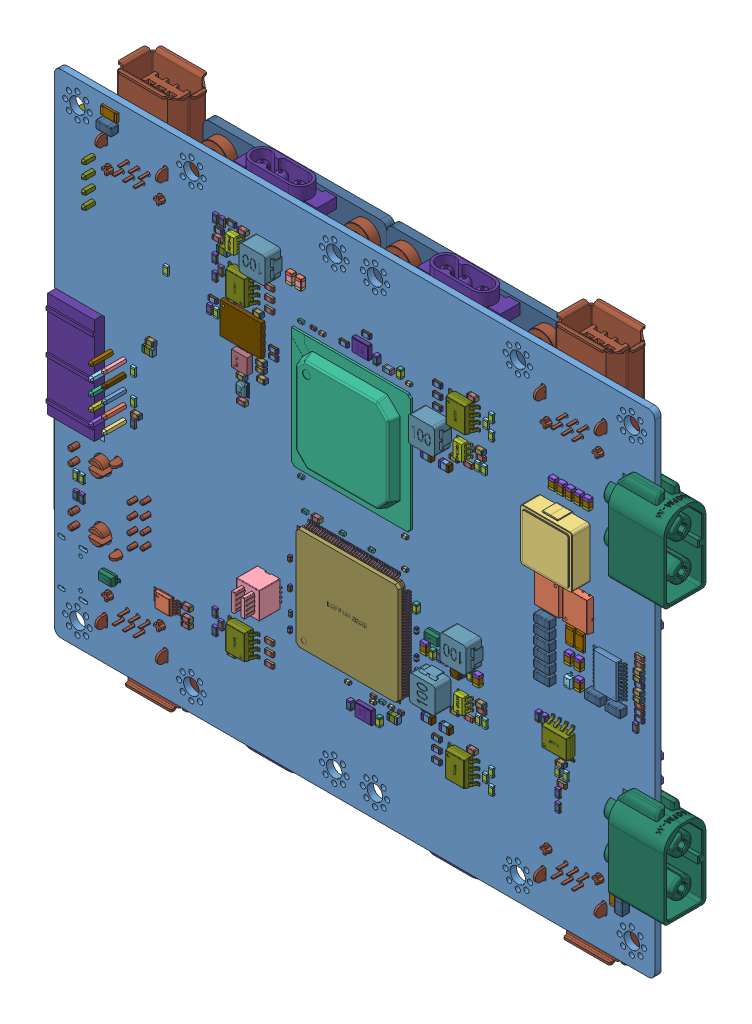
SolidWorks assembly Mother  Board, configuration 默认. Lengths in mm. (continued)
Components (placement in the parent): (continued)
- Mother  Board.step-1: Mother  Board.step [默认] at origin size (122.6 102.08 21) (continued)
  - R56.step-1: R56.step [默认] at origin size (0.5 1 0.35)
    - 5993847584.step-1: 5993847584.step [默认] at (46.4669 57.4279 -1.2164) x (0 -1 0) z (0 0 -1) size (1 0.5 0.35)
      - Terminal-11.step-1: Terminal-11.step [默认] at (-0.5 -0.25 0) size (0.25 0.5 0.35)
        - Open_CASCADE_STEP_translator_6.8_20.2.1-25.step-1: Open_CASCADE_STEP_translator_6.8_20.2.1-25.step [默认] at origin size (0.25 0.5 0.35)
      - Terminal-11.step-2: Terminal-11.step [默认] at (0.5 0.25 0) x (-1 0 0) z (0 0 1) size (0.25 0.5 0.35)
        - Open_CASCADE_STEP_translator_6.8_20.2.1-25.step-1: Open_CASCADE_STEP_translator_6.8_20.2.1-25.step [默认] at origin size (0.25 0.5 0.35)
      - Mid_Body-26.step-1: Mid_Body-26.step [默认] at (-0.5 -0.25 0) size (0.93 0.5 0.28)
      - Mark-27.step-1: Mark-27.step [默认] at (-0.25 -0.25 0.315) size (0.5 0.5 0.03)
  - R55.step-1: R55.step [默认] at origin size (1 0.5 0.35)
    - 5993847504.step-1: 5993847504.step [默认] at (44.9669 62.9361 -1.2164) x (-1 0 0) z (0 0 -1) size (1 0.5 0.35)
      - Terminal-8.step-1: Terminal-8.step [默认] at (-0.5 -0.25 0) size (0.25 0.5 0.35)
        - Open_CASCADE_STEP_translator_6.8_20.2.1-16.step-1: Open_CASCADE_STEP_translator_6.8_20.2.1-16.step [默认] at origin size (0.25 0.5 0.35)
      - Terminal-8.step-2: Terminal-8.step [默认] at (0.5 0.25 0) x (-1 0 0) z (0 0 1) size (0.25 0.5 0.35)
        - Open_CASCADE_STEP_translator_6.8_20.2.1-16.step-1: Open_CASCADE_STEP_translator_6.8_20.2.1-16.step [默认] at origin size (0.25 0.5 0.35)
      - Mid_Body-17.step-1: Mid_Body-17.step [默认] at (-0.5 -0.25 0) size (0.93 0.5 0.28)
      - Mark-18.step-1: Mark-18.step [默认] at (-0.25 -0.25 0.315) size (0.5 0.5 0.03)
  - R54.step-1: R54.step [默认] at origin size (0.5 1 0.35)
    - 5993847584.step-1: 5993847584.step [默认] at (60.4669 57.4279 -1.2164) x (0 -1 0) z (0 0 -1) size (1 0.5 0.35)
      - Terminal-11.step-1: Terminal-11.step [默认] at (-0.5 -0.25 0) size (0.25 0.5 0.35)
        - Open_CASCADE_STEP_translator_6.8_20.2.1-25.step-1: Open_CASCADE_STEP_translator_6.8_20.2.1-25.step [默认] at origin size (0.25 0.5 0.35)
      - Terminal-11.step-2: Terminal-11.step [默认] at (0.5 0.25 0) x (-1 0 0) z (0 0 1) size (0.25 0.5 0.35)
        - Open_CASCADE_STEP_translator_6.8_20.2.1-25.step-1: Open_CASCADE_STEP_translator_6.8_20.2.1-25.step [默认] at origin size (0.25 0.5 0.35)
      - Mid_Body-26.step-1: Mid_Body-26.step [默认] at (-0.5 -0.25 0) size (0.93 0.5 0.28)
      - Mark-27.step-1: Mark-27.step [默认] at (-0.25 -0.25 0.315) size (0.5 0.5 0.03)
  - R53.step-1: R53.step [默认] at origin size (1.6 0.8 0.45)
    - 5993842144.step-1: 5993842144.step [默认] at (38.1001 64.5161 0) x (1 0 0) z (0 0 1) size (1.6 0.8 0.45)
      - Terminal-10.step-1: Terminal-10.step [默认] at (-0.8 -0.4 0) size (0.3 0.8 0.45)
        - Open_CASCADE_STEP_translator_6.8_21.2.1-22.step-1: Open_CASCADE_STEP_translator_6.8_21.2.1-22.step [默认] at origin size (0.3 0.8 0.45)
      - Terminal-10.step-2: Terminal-10.step [默认] at (0.8 0.4 0) x (-1 0 0) z (0 0 1) size (0.3 0.8 0.45)
        - Open_CASCADE_STEP_translator_6.8_21.2.1-22.step-1: Open_CASCADE_STEP_translator_6.8_21.2.1-22.step [默认] at origin size (0.3 0.8 0.45)
      - Mid_Body-23.step-1: Mid_Body-23.step [默认] at (-0.8 -0.4 0) size (1.51 0.8 0.36)
      - Mark-24.step-1: Mark-24.step [默认] at (-0.5 -0.4 0.405) size (1 0.8 0.05)
  - R52.step-1: R52.step [默认] at origin size (0.8 1.6 0.45)
    - 5993842864.step-1: 5993842864.step [默认] at (27.0509 65.1511 0) x (0 1 0) z (0 0 1) size (1.6 0.8 0.45)
      - Terminal-12.step-1: Terminal-12.step [默认] at (-0.8 -0.4 0) size (0.3 0.8 0.45)
        - Open_CASCADE_STEP_translator_6.8_21.2.1-28.step-1: Open_CASCADE_STEP_translator_6.8_21.2.1-28.step [默认] at origin size (0.3 0.8 0.45)
      - Terminal-12.step-2: Terminal-12.step [默认] at (0.8 0.4 0) x (-1 0 0) z (0 0 1) size (0.3 0.8 0.45)
        - Open_CASCADE_STEP_translator_6.8_21.2.1-28.step-1: Open_CASCADE_STEP_translator_6.8_21.2.1-28.step [默认] at origin size (0.3 0.8 0.45)
      - Mid_Body-29.step-1: Mid_Body-29.step [默认] at (-0.8 -0.4 0) size (1.51 0.8 0.36)
      - Mark-30.step-1: Mark-30.step [默认] at (-0.5 -0.4 0.405) size (1 0.8 0.05)
  - R51.step-1: R51.step [默认] at origin size (0.8 1.6 0.45)
    - 5993843024.step-1: 5993843024.step [默认] at (11.0491 38.7349 0) x (0 -1 0) z (0 0 1) size (1.6 0.8 0.45)
      - Terminal-13.step-1: Terminal-13.step [默认] at (-0.8 -0.4 0) size (0.3 0.8 0.45)
        - Open_CASCADE_STEP_translator_6.8_21.2.1-31.step-1: Open_CASCADE_STEP_translator_6.8_21.2.1-31.step [默认] at origin size (0.3 0.8 0.45)
      - Terminal-13.step-2: Terminal-13.step [默认] at (0.8 0.4 0) x (-1 0 0) z (0 0 1) size (0.3 0.8 0.45)
        - Open_CASCADE_STEP_translator_6.8_21.2.1-31.step-1: Open_CASCADE_STEP_translator_6.8_21.2.1-31.step [默认] at origin size (0.3 0.8 0.45)
      - Mid_Body-32.step-1: Mid_Body-32.step [默认] at (-0.8 -0.4 0) size (1.51 0.8 0.36)
      - Mark-33.step-1: Mark-33.step [默认] at (-0.5 -0.4 0.405) size (1 0.8 0.05)
  - R50.step-1: R50.step [默认] at origin size (0.8 1.6 0.45)
    - 5993842864.step-1: 5993842864.step [默认] at (11.0489 42.2911 0) x (0 1 0) z (0 0 1) size (1.6 0.8 0.45)
      - Terminal-12.step-1: Terminal-12.step [默认] at (-0.8 -0.4 0) size (0.3 0.8 0.45)
        - Open_CASCADE_STEP_translator_6.8_21.2.1-28.step-1: Open_CASCADE_STEP_translator_6.8_21.2.1-28.step [默认] at origin size (0.3 0.8 0.45)
      - Terminal-12.step-2: Terminal-12.step [默认] at (0.8 0.4 0) x (-1 0 0) z (0 0 1) size (0.3 0.8 0.45)
        - Open_CASCADE_STEP_translator_6.8_21.2.1-28.step-1: Open_CASCADE_STEP_translator_6.8_21.2.1-28.step [默认] at origin size (0.3 0.8 0.45)
      - Mid_Body-29.step-1: Mid_Body-29.step [默认] at (-0.8 -0.4 0) size (1.51 0.8 0.36)
      - Mark-30.step-1: Mark-30.step [默认] at (-0.5 -0.4 0.405) size (1 0.8 0.05)
  - R49.step-1: R49.step [默认] at origin size (1.6 0.8 0.45)
    - 5993842144.step-1: 5993842144.step [默认] at (38.1001 63.2461 0) x (1 0 0) z (0 0 1) size (1.6 0.8 0.45)
      - Terminal-10.step-1: Terminal-10.step [默认] at (-0.8 -0.4 0) size (0.3 0.8 0.45)
        - Open_CASCADE_STEP_translator_6.8_21.2.1-22.step-1: Open_CASCADE_STEP_translator_6.8_21.2.1-22.step [默认] at origin size (0.3 0.8 0.45)
      - Terminal-10.step-2: Terminal-10.step [默认] at (0.8 0.4 0) x (-1 0 0) z (0 0 1) size (0.3 0.8 0.45)
        - Open_CASCADE_STEP_translator_6.8_21.2.1-22.step-1: Open_CASCADE_STEP_translator_6.8_21.2.1-22.step [默认] at origin size (0.3 0.8 0.45)
      - Mid_Body-23.step-1: Mid_Body-23.step [默认] at (-0.8 -0.4 0) size (1.51 0.8 0.36)
      - Mark-24.step-1: Mark-24.step [默认] at (-0.5 -0.4 0.405) size (1 0.8 0.05)
  - R48.step-1: R48.step [默认] at origin size (1.6 0.8 0.45)
    - 5993842144.step-1: 5993842144.step [默认] at (26.4161 67.0561 0) x (1 0 0) z (0 0 1) size (1.6 0.8 0.45)
      - Terminal-10.step-1: Terminal-10.step [默认] at (-0.8 -0.4 0) size (0.3 0.8 0.45)
        - Open_CASCADE_STEP_translator_6.8_21.2.1-22.step-1: Open_CASCADE_STEP_translator_6.8_21.2.1-22.step [默认] at origin size (0.3 0.8 0.45)
      - Terminal-10.step-2: Terminal-10.step [默认] at (0.8 0.4 0) x (-1 0 0) z (0 0 1) size (0.3 0.8 0.45)
        - Open_CASCADE_STEP_translator_6.8_21.2.1-22.step-1: Open_CASCADE_STEP_translator_6.8_21.2.1-22.step [默认] at origin size (0.3 0.8 0.45)
      - Mid_Body-23.step-1: Mid_Body-23.step [默认] at (-0.8 -0.4 0) size (1.51 0.8 0.36)
      - Mark-24.step-1: Mark-24.step [默认] at (-0.5 -0.4 0.405) size (1 0.8 0.05)
  - R47.step-1: R47.step [默认] at origin size (0.8 1.6 0.45)
    - 5993843024.step-1: 5993843024.step [默认] at (25.7811 65.1509 0) x (0 -1 0) z (0 0 1) size (1.6 0.8 0.45)
      - Terminal-13.step-1: Terminal-13.step [默认] at (-0.8 -0.4 0) size (0.3 0.8 0.45)
        - Open_CASCADE_STEP_translator_6.8_21.2.1-31.step-1: Open_CASCADE_STEP_translator_6.8_21.2.1-31.step [默认] at origin size (0.3 0.8 0.45)
      - Terminal-13.step-2: Terminal-13.step [默认] at (0.8 0.4 0) x (-1 0 0) z (0 0 1) size (0.3 0.8 0.45)
        - Open_CASCADE_STEP_translator_6.8_21.2.1-31.step-1: Open_CASCADE_STEP_translator_6.8_21.2.1-31.step [默认] at origin size (0.3 0.8 0.45)
      - Mid_Body-32.step-1: Mid_Body-32.step [默认] at (-0.8 -0.4 0) size (1.51 0.8 0.36)
      - Mark-33.step-1: Mark-33.step [默认] at (-0.5 -0.4 0.405) size (1 0.8 0.05)
  - R46.step-1: R46.step [默认] at origin size (0.8 1.6 0.45)
    - 5993842864.step-1: 5993842864.step [默认] at (11.0489 47.3711 0) x (0 1 0) z (0 0 1) size (1.6 0.8 0.45)
      - Terminal-12.step-1: Terminal-12.step [默认] at (-0.8 -0.4 0) size (0.3 0.8 0.45)
        - Open_CASCADE_STEP_translator_6.8_21.2.1-28.step-1: Open_CASCADE_STEP_translator_6.8_21.2.1-28.step [默认] at origin size (0.3 0.8 0.45)
      - Terminal-12.step-2: Terminal-12.step [默认] at (0.8 0.4 0) x (-1 0 0) z (0 0 1) size (0.3 0.8 0.45)
        - Open_CASCADE_STEP_translator_6.8_21.2.1-28.step-1: Open_CASCADE_STEP_translator_6.8_21.2.1-28.step [默认] at origin size (0.3 0.8 0.45)
      - Mid_Body-29.step-1: Mid_Body-29.step [默认] at (-0.8 -0.4 0) size (1.51 0.8 0.36)
      - Mark-30.step-1: Mark-30.step [默认] at (-0.5 -0.4 0.405) size (1 0.8 0.05)
  - R25.step-1: R25.step [默认] at origin size (1.6 0.8 0.45)
    - 5993842944.step-1: 5993842944.step [默认] at (75.6919 64.1349 0) x (-1 0 0) z (0 0 1) size (1.6 0.8 0.45)
      - Terminal-14.step-1: Terminal-14.step [默认] at (-0.8 -0.4 0) size (0.3 0.8 0.45)
        - Open_CASCADE_STEP_translator_6.8_21.2.1-34.step-1: Open_CASCADE_STEP_translator_6.8_21.2.1-34.step [默认] at origin size (0.3 0.8 0.45)
      - Terminal-14.step-2: Terminal-14.step [默认] at (0.8 0.4 0) x (-1 0 0) z (0 0 1) size (0.3 0.8 0.45)
        - Open_CASCADE_STEP_translator_6.8_21.2.1-34.step-1: Open_CASCADE_STEP_translator_6.8_21.2.1-34.step [默认] at origin size (0.3 0.8 0.45)
      - Mid_Body-35.step-1: Mid_Body-35.step [默认] at (-0.8 -0.4 0) size (1.51 0.8 0.36)
      - Mark-36.step-1: Mark-36.step [默认] at (-0.5 -0.4 0.405) size (1 0.8 0.05)
  - R24.step-1: R24.step [默认] at origin size (1.6 0.8 0.45)
    - 5993842144.step-1: 5993842144.step [默认] at (29.9721 81.5341 0) x (1 0 0) z (0 0 1) size (1.6 0.8 0.45)
      - Terminal-10.step-1: Terminal-10.step [默认] at (-0.8 -0.4 0) size (0.3 0.8 0.45)
        - Open_CASCADE_STEP_translator_6.8_21.2.1-22.step-1: Open_CASCADE_STEP_translator_6.8_21.2.1-22.step [默认] at origin size (0.3 0.8 0.45)
      - Terminal-10.step-2: Terminal-10.step [默认] at (0.8 0.4 0) x (-1 0 0) z (0 0 1) size (0.3 0.8 0.45)
        - Open_CASCADE_STEP_translator_6.8_21.2.1-22.step-1: Open_CASCADE_STEP_translator_6.8_21.2.1-22.step [默认] at origin size (0.3 0.8 0.45)
      - Mid_Body-23.step-1: Mid_Body-23.step [默认] at (-0.8 -0.4 0) size (1.51 0.8 0.36)
      - Mark-24.step-1: Mark-24.step [默认] at (-0.5 -0.4 0.405) size (1 0.8 0.05)
  - R23.step-1: R23.step [默认] at origin size (1.6 0.8 0.45)
    - 5993842944.step-1: 5993842944.step [默认] at (75.8189 21.8439 0) x (-1 0 0) z (0 0 1) size (1.6 0.8 0.45)
      - Terminal-14.step-1: Terminal-14.step [默认] at (-0.8 -0.4 0) size (0.3 0.8 0.45)
        - Open_CASCADE_STEP_translator_6.8_21.2.1-34.step-1: Open_CASCADE_STEP_translator_6.8_21.2.1-34.step [默认] at origin size (0.3 0.8 0.45)
      - Terminal-14.step-2: Terminal-14.step [默认] at (0.8 0.4 0) x (-1 0 0) z (0 0 1) size (0.3 0.8 0.45)
        - Open_CASCADE_STEP_translator_6.8_21.2.1-34.step-1: Open_CASCADE_STEP_translator_6.8_21.2.1-34.step [默认] at origin size (0.3 0.8 0.45)
      - Mid_Body-35.step-1: Mid_Body-35.step [默认] at (-0.8 -0.4 0) size (1.51 0.8 0.36)
      - Mark-36.step-1: Mark-36.step [默认] at (-0.5 -0.4 0.405) size (1 0.8 0.05)
  - R22.step-1: R22.step [默认] at origin size (0.8 1.6 0.45)
    - 5993842864.step-1: 5993842864.step [默认] at (77.4699 64.7701 0) x (0 1 0) z (0 0 1) size (1.6 0.8 0.45)
      - Terminal-12.step-1: Terminal-12.step [默认] at (-0.8 -0.4 0) size (0.3 0.8 0.45)
        - Open_CASCADE_STEP_translator_6.8_21.2.1-28.step-1: Open_CASCADE_STEP_translator_6.8_21.2.1-28.step [默认] at origin size (0.3 0.8 0.45)
      - Terminal-12.step-2: Terminal-12.step [默认] at (0.8 0.4 0) x (-1 0 0) z (0 0 1) size (0.3 0.8 0.45)
        - Open_CASCADE_STEP_translator_6.8_21.2.1-28.step-1: Open_CASCADE_STEP_translator_6.8_21.2.1-28.step [默认] at origin size (0.3 0.8 0.45)
      - Mid_Body-29.step-1: Mid_Body-29.step [默认] at (-0.8 -0.4 0) size (1.51 0.8 0.36)
      - Mark-30.step-1: Mark-30.step [默认] at (-0.5 -0.4 0.405) size (1 0.8 0.05)
  - R21.step-1: R21.step [默认] at origin size (0.8 1.6 0.45)
    - 5993843024.step-1: 5993843024.step [默认] at (28.1941 80.8989 0) x (0 -1 0) z (0 0 1) size (1.6 0.8 0.45)
      - Terminal-13.step-1: Terminal-13.step [默认] at (-0.8 -0.4 0) size (0.3 0.8 0.45)
        - Open_CASCADE_STEP_translator_6.8_21.2.1-31.step-1: Open_CASCADE_STEP_translator_6.8_21.2.1-31.step [默认] at origin size (0.3 0.8 0.45)
      - Terminal-13.step-2: Terminal-13.step [默认] at (0.8 0.4 0) x (-1 0 0) z (0 0 1) size (0.3 0.8 0.45)
        - Open_CASCADE_STEP_translator_6.8_21.2.1-31.step-1: Open_CASCADE_STEP_translator_6.8_21.2.1-31.step [默认] at origin size (0.3 0.8 0.45)
      - Mid_Body-32.step-1: Mid_Body-32.step [默认] at (-0.8 -0.4 0) size (1.51 0.8 0.36)
      - Mark-33.step-1: Mark-33.step [默认] at (-0.5 -0.4 0.405) size (1 0.8 0.05)
  - R20.step-1: R20.step [默认] at origin size (0.8 1.6 0.45)
    - 5993842864.step-1: 5993842864.step [默认] at (77.5969 22.4791 0) x (0 1 0) z (0 0 1) size (1.6 0.8 0.45)
      - Terminal-12.step-1: Terminal-12.step [默认] at (-0.8 -0.4 0) size (0.3 0.8 0.45)
        - Open_CASCADE_STEP_translator_6.8_21.2.1-28.step-1: Open_CASCADE_STEP_translator_6.8_21.2.1-28.step [默认] at origin size (0.3 0.8 0.45)
      - Terminal-12.step-2: Terminal-12.step [默认] at (0.8 0.4 0) x (-1 0 0) z (0 0 1) size (0.3 0.8 0.45)
        - Open_CASCADE_STEP_translator_6.8_21.2.1-28.step-1: Open_CASCADE_STEP_translator_6.8_21.2.1-28.step [默认] at origin size (0.3 0.8 0.45)
      - Mid_Body-29.step-1: Mid_Body-29.step [默认] at (-0.8 -0.4 0) size (1.51 0.8 0.36)
      - Mark-30.step-1: Mark-30.step [默认] at (-0.5 -0.4 0.405) size (1 0.8 0.05)
  - R19.step-1: R19.step [默认] at origin size (0.8 1.6 0.45)
    - 5993842864.step-1: 5993842864.step [默认] at (78.7399 64.7701 0) x (0 1 0) z (0 0 1) size (1.6 0.8 0.45)
      - Terminal-12.step-1: Terminal-12.step [默认] at (-0.8 -0.4 0) size (0.3 0.8 0.45)
        - Open_CASCADE_STEP_translator_6.8_21.2.1-28.step-1: Open_CASCADE_STEP_translator_6.8_21.2.1-28.step [默认] at origin size (0.3 0.8 0.45)
      - Terminal-12.step-2: Terminal-12.step [默认] at (0.8 0.4 0) x (-1 0 0) z (0 0 1) size (0.3 0.8 0.45)
        - Open_CASCADE_STEP_translator_6.8_21.2.1-28.step-1: Open_CASCADE_STEP_translator_6.8_21.2.1-28.step [默认] at origin size (0.3 0.8 0.45)
      - Mid_Body-29.step-1: Mid_Body-29.step [默认] at (-0.8 -0.4 0) size (1.51 0.8 0.36)
      - Mark-30.step-1: Mark-30.step [默认] at (-0.5 -0.4 0.405) size (1 0.8 0.05)
  - R18.step-1: R18.step [默认] at origin size (0.8 1.6 0.45)
    - 5993843024.step-1: 5993843024.step [默认] at (26.9241 80.8989 0) x (0 -1 0) z (0 0 1) size (1.6 0.8 0.45)
      - Terminal-13.step-1: Terminal-13.step [默认] at (-0.8 -0.4 0) size (0.3 0.8 0.45)
        - Open_CASCADE_STEP_translator_6.8_21.2.1-31.step-1: Open_CASCADE_STEP_translator_6.8_21.2.1-31.step [默认] at origin size (0.3 0.8 0.45)
      - Terminal-13.step-2: Terminal-13.step [默认] at (0.8 0.4 0) x (-1 0 0) z (0 0 1) size (0.3 0.8 0.45)
        - Open_CASCADE_STEP_translator_6.8_21.2.1-31.step-1: Open_CASCADE_STEP_translator_6.8_21.2.1-31.step [默认] at origin size (0.3 0.8 0.45)
      - Mid_Body-32.step-1: Mid_Body-32.step [默认] at (-0.8 -0.4 0) size (1.51 0.8 0.36)
      - Mark-33.step-1: Mark-33.step [默认] at (-0.5 -0.4 0.405) size (1 0.8 0.05)
  - R17.step-1: R17.step [默认] at origin size (0.8 1.6 0.45)
    - 5993842864.step-1: 5993842864.step [默认] at (78.8669 22.4791 0) x (0 1 0) z (0 0 1) size (1.6 0.8 0.45)
      - Terminal-12.step-1: Terminal-12.step [默认] at (-0.8 -0.4 0) size (0.3 0.8 0.45)
        - Open_CASCADE_STEP_translator_6.8_21.2.1-28.step-1: Open_CASCADE_STEP_translator_6.8_21.2.1-28.step [默认] at origin size (0.3 0.8 0.45)
      - Terminal-12.step-2: Terminal-12.step [默认] at (0.8 0.4 0) x (-1 0 0) z (0 0 1) size (0.3 0.8 0.45)
        - Open_CASCADE_STEP_translator_6.8_21.2.1-28.step-1: Open_CASCADE_STEP_translator_6.8_21.2.1-28.step [默认] at origin size (0.3 0.8 0.45)
      - Mid_Body-29.step-1: Mid_Body-29.step [默认] at (-0.8 -0.4 0) size (1.51 0.8 0.36)
      - Mark-30.step-1: Mark-30.step [默认] at (-0.5 -0.4 0.405) size (1 0.8 0.05)
  - R16.step-1: R16.step [默认] at origin size (1.6 0.8 0.45)
    - 5993842944.step-1: 5993842944.step [默认] at (78.1049 66.5479 0) x (-1 0 0) z (0 0 1) size (1.6 0.8 0.45)
      - Terminal-14.step-1: Terminal-14.step [默认] at (-0.8 -0.4 0) size (0.3 0.8 0.45)
        - Open_CASCADE_STEP_translator_6.8_21.2.1-34.step-1: Open_CASCADE_STEP_translator_6.8_21.2.1-34.step [默认] at origin size (0.3 0.8 0.45)
      - Terminal-14.step-2: Terminal-14.step [默认] at (0.8 0.4 0) x (-1 0 0) z (0 0 1) size (0.3 0.8 0.45)
        - Open_CASCADE_STEP_translator_6.8_21.2.1-34.step-1: Open_CASCADE_STEP_translator_6.8_21.2.1-34.step [默认] at origin size (0.3 0.8 0.45)
      - Mid_Body-35.step-1: Mid_Body-35.step [默认] at (-0.8 -0.4 0) size (1.51 0.8 0.36)
      - Mark-36.step-1: Mark-36.step [默认] at (-0.5 -0.4 0.405) size (1 0.8 0.05)
  - R15.step-1: R15.step [默认] at origin size (1.6 0.8 0.45)
    - 5993842144.step-1: 5993842144.step [默认] at (27.5591 79.1211 0) x (1 0 0) z (0 0 1) size (1.6 0.8 0.45)
      - Terminal-10.step-1: Terminal-10.step [默认] at (-0.8 -0.4 0) size (0.3 0.8 0.45)
        - Open_CASCADE_STEP_translator_6.8_21.2.1-22.step-1: Open_CASCADE_STEP_translator_6.8_21.2.1-22.step [默认] at origin size (0.3 0.8 0.45)
      - Terminal-10.step-2: Terminal-10.step [默认] at (0.8 0.4 0) x (-1 0 0) z (0 0 1) size (0.3 0.8 0.45)
        - Open_CASCADE_STEP_translator_6.8_21.2.1-22.step-1: Open_CASCADE_STEP_translator_6.8_21.2.1-22.step [默认] at origin size (0.3 0.8 0.45)
      - Mid_Body-23.step-1: Mid_Body-23.step [默认] at (-0.8 -0.4 0) size (1.51 0.8 0.36)
      - Mark-24.step-1: Mark-24.step [默认] at (-0.5 -0.4 0.405) size (1 0.8 0.05)
  - R14.step-1: R14.step [默认] at origin size (1.6 0.8 0.45)
    - 5993842944.step-1: 5993842944.step [默认] at (78.2319 24.2569 0) x (-1 0 0) z (0 0 1) size (1.6 0.8 0.45)
      - Terminal-14.step-1: Terminal-14.step [默认] at (-0.8 -0.4 0) size (0.3 0.8 0.45)
        - Open_CASCADE_STEP_translator_6.8_21.2.1-34.step-1: Open_CASCADE_STEP_translator_6.8_21.2.1-34.step [默认] at origin size (0.3 0.8 0.45)
      - Terminal-14.step-2: Terminal-14.step [默认] at (0.8 0.4 0) x (-1 0 0) z (0 0 1) size (0.3 0.8 0.45)
        - Open_CASCADE_STEP_translator_6.8_21.2.1-34.step-1: Open_CASCADE_STEP_translator_6.8_21.2.1-34.step [默认] at origin size (0.3 0.8 0.45)
      - Mid_Body-35.step-1: Mid_Body-35.step [默认] at (-0.8 -0.4 0) size (1.51 0.8 0.36)
      - Mark-36.step-1: Mark-36.step [默认] at (-0.5 -0.4 0.405) size (1 0.8 0.05)
  - L4.step-1: L4.step [默认] at origin size (5.6 5 3.1)
    - User_Library-FERROCORE_HPI0530-100.step-1: User_Library-FERROCORE_HPI0530-100.step [默认] at (71.8419 64.6329 0) x (1 0 0) z (0 -1 0) size (5.6 3.1 5)
  - L3.step-1: L3.step [默认] at origin size (5.6 5 3.1)
    - User_Library-FERROCORE_HPI0530-100.step-1: User_Library-FERROCORE_HPI0530-100.step [默认] at (34.2031 81.9251 0) x (-1 0 0) z (0 1 0) size (5.6 3.1 5)
  - L2.step-1: L2.step [默认] at origin size (5 5.6 3.1)
    - User_Library-FERROCORE_HPI0530-100.step-1: User_Library-FERROCORE_HPI0530-100.step [默认] at (72.0191 26.5029 0) x (0 1 0) z (1 0 0) size (5.6 3.1 5)
  - JP7.step-1: JP7.step [默认] at origin size (7.7 12.62 9.1)
    - XH2.54-4P_H.step-1: XH2.54-4P_H.step [默认] at (3.048 71.501 -1.2464) x (0 1 0) z (-1 0 0) size (12.62 9.1 7.7)
      - LOGO_.step-1: LOGO_.step [默认] at (-1.159 -0.003 2.4494) x (0 0 1) z (0 -1 0) size (0.9 1.04 0.01)
      - XH2.54-4P_H-37.step-1: XH2.54-4P_H-37.step [默认] at origin size (12.62 9.1 7.7)
  - JP6.step-1: JP6.step [默认] at origin size (13.8 20.3 12)
    - User_Library-DC3-10P.step-1: User_Library-DC3-10P.step [默认] at (-4.4451 43.0529 1.2836) x (0 1 0) z (-1 0 0) size (20.3 12 13.8)
      - unnamed.step-1: unnamed.step [默认] at origin size (20.3 9.4 9)
      - unnamed-38.step-1: unnamed-38.step [默认] at origin size (0.64 9.04 12.8)
      - unnamed-39.step-1: unnamed-39.step [默认] at origin size (0.64 9.04 12.8)
      - unnamed-40.step-1: unnamed-40.step [默认] at origin size (0.64 9.04 12.8)
      - unnamed-41.step-1: unnamed-41.step [默认] at origin size (0.64 9.04 12.8)
      - unnamed-42.step-1: unnamed-42.step [默认] at origin size (0.64 9.04 12.8)
      - unnamed-43.step-1: unnamed-43.step [默认] at origin size (0.64 6.5 10.26)
      - unnamed-44.step-1: unnamed-44.step [默认] at origin size (0.64 6.5 10.26)
      - unnamed-45.step-1: unnamed-45.step [默认] at origin size (0.64 6.5 10.26)
      - unnamed-46.step-1: unnamed-46.step [默认] at origin size (0.64 6.5 10.26)
      - unnamed-47.step-1: unnamed-47.step [默认] at origin size (0.64 6.5 10.26)
  - JP2_D3.step-1: JP2_D3.step [默认] at origin size (11.5 5 4.6)
    - SG340-GxxS-B1-2x12.step-1: SG340-GxxS-B1-2x12.step [默认] at (35.7506 47.117 -1.3164) x (-1 0 0) z (0 0 -1) size (11.5 5 4.6)
  - JP2_D2.step-1: JP2_D2.step [默认] at origin size (11.5 5 4.6)
    - SG340-GxxS-B1-2x12.step-1: SG340-GxxS-B1-2x12.step [默认] at (71.1834 38.989 -1.3164) x (1 0 0) z (0 0 -1) size (11.5 5 4.6)
  - JP2_D1.step-1: JP2_D1.step [默认] at origin size (11.5 5 4.6)
    - SG340-GxxS-B1-2x12.step-1: SG340-GxxS-B1-2x12.step [默认] at (35.7504 38.989 -1.3164) x (1 0 0) z (0 0 -1) size (11.5 5 4.6)
  - JP1_D3.step-1: JP1_D3.step [默认] at origin size (13.5 16.6 11.9)
    - 1364-6.step-1: 1364-6.step [默认] at (11.1678 94.092 -5.9164) x (1 0 0) z (0 1 0) size (13.5 11.9 16.6)
  - JP1_D2.step-1: JP1_D2.step [默认] at origin size (13.5 16.6 11.9)
    - 1364-6.step-1: 1364-6.step [默认] at (95.7662 -7.986 -5.9164) x (-1 0 0) z (0 -1 0) size (13.5 11.9 16.6)
  - JP1_D1.step-1: JP1_D1.step [默认] at origin size (13.5 16.6 11.9)
    - 1364-6.step-1: 1364-6.step [默认] at (11.168 -7.986 -5.9164) x (-1 0 0) z (0 -1 0) size (13.5 11.9 16.6)
  - FB2.step-1: FB2.step [默认] at origin size (1.6 0.8 0.8)
    - 742792606.step-1: 742792606.step [默认] at (60.4519 72.3899 0.39) x (0 -1 0) z (0 0 1) size (0.8 0.3 0.8)
    - 742792606-48.step-1: 742792606-48.step [默认] at (60.4519 72.3899 0.39) x (0 -1 0) z (0 0 1) size (0.8 0.3 0.8)
    - 742792606-49.step-1: 742792606-49.step [默认] at (60.4519 72.3899 0.39) x (0 -1 0) z (0 0 1) size (0.8 1 0.8)
  - D3.step-1: D3.step [默认] at origin size (3.7 1.6 1.22)
    - SOD-123.step-1: SOD-123.step [默认] at (6.477 10.795 0.05) x (-1 0 0) z (0 0 1) size (3.7 1.6 1.22)
      - SOD-123-50.step-1: SOD-123-50.step [默认] at origin size (3.7 1.6 1.22)
      - LOGO______.__.step-1: LOGO______.__.step [默认] at (-0.0155 0.0364 -0.003) x (-1 0 0) z (0 0 -1) size (0.9 1.04 0.01)
  - C57.step-1: C57.step [默认] at origin size (1 0.5 0.5)
    - 5993845104.step-1: 5993845104.step [默认] at (47.4979 71.8819 0) x (-1 0 0) z (0 0 1) size (1 0.5 0.5)
      - Terminal-3.step-1: Terminal-3.step [默认] at (-0.5 -0.25 0) size (1 0.5 0.5)
        - Open_CASCADE_STEP_translator_6.8_54.1.1-1.step-1: Open_CASCADE_STEP_translator_6.8_54.1.1-1.step [默认] at origin size (0.25 0.5 0.5)
        - Open_CASCADE_STEP_translator_6.8_54.1.2-2.step-1: Open_CASCADE_STEP_translator_6.8_54.1.2-2.step [默认] at origin size (0.25 0.5 0.5)
      - Mid_Body-2.step-1: Mid_Body-2.step [默认] at (-0.5 -0.25 0) size (0.5 0.5 0.5)
        - Open_CASCADE_STEP_translator_6.8_54.2.1-3.step-1: Open_CASCADE_STEP_translator_6.8_54.2.1-3.step [默认] at origin size (0.5 0.5 0.5)
  - C22.step-1: C22.step [默认] at origin size (2.01 1.25 0.94)
    - 5993850784.step-1: 5993850784.step [默认] at (68.0721 61.9761 0) x (1 0 0) z (0 0 1) size (2.01 1.25 0.94)
      - Fillet1.step-1: Fillet1.step [默认] at origin size (0.5 1.25 0.94)
      - Fillet2.step-1: Fillet2.step [默认] at origin size (0.5 1.25 0.94)
      - body2.step-1: body2.step [默认] at origin size (1.01 1.22 0.92)
  - C20.step-1: C20.step [默认] at origin size (1.25 2.01 0.94)
    - 5993850384.step-1: 5993850384.step [默认] at (41.6561 78.4859 0) x (0 -1 0) z (0 0 1) size (2.01 1.25 0.94)
      - Fillet1-51.step-1: Fillet1-51.step [默认] at origin size (0.5 1.25 0.94)
      - Fillet2-52.step-1: Fillet2-52.step [默认] at origin size (0.5 1.25 0.94)
      - body2-53.step-1: body2-53.step [默认] at origin size (1.01 1.22 0.92)
  - C18.step-1: C18.step [默认] at origin size (2.01 1.25 0.94)
    - 5993850784.step-1: 5993850784.step [默认] at (68.1991 19.8121 0) x (1 0 0) z (0 0 1) size (2.01 1.25 0.94)
      - Fillet1.step-1: Fillet1.step [默认] at origin size (0.5 1.25 0.94)
      - Fillet2.step-1: Fillet2.step [默认] at origin size (0.5 1.25 0.94)
      - body2.step-1: body2.step [默认] at origin size (1.01 1.22 0.92)
  - C144.step-1: C144.step [默认] at origin size (1 0.5 0.5)
    - 5993845104.step-1: 5993845104.step [默认] at (57.2769 15.2399 0) x (-1 0 0) z (0 0 1) size (1 0.5 0.5)
      - Terminal-3.step-1: Terminal-3.step [默认] at (-0.5 -0.25 0) size (1 0.5 0.5)
        - Open_CASCADE_STEP_translator_6.8_54.1.1-1.step-1: Open_CASCADE_STEP_translator_6.8_54.1.1-1.step [默认] at origin size (0.25 0.5 0.5)
        - Open_CASCADE_STEP_translator_6.8_54.1.2-2.step-1: Open_CASCADE_STEP_translator_6.8_54.1.2-2.step [默认] at origin size (0.25 0.5 0.5)
      - Mid_Body-2.step-1: Mid_Body-2.step [默认] at (-0.5 -0.25 0) size (0.5 0.5 0.5)
        - Open_CASCADE_STEP_translator_6.8_54.2.1-3.step-1: Open_CASCADE_STEP_translator_6.8_54.2.1-3.step [默认] at origin size (0.5 0.5 0.5)
  - C143.step-1: C143.step [默认] at origin size (0.8 1.6 0.8)
    - 5993853744.step-1: 5993853744.step [默认] at (58.6739 12.8271 0) x (0 1 0) z (0 0 1) size (1.6 0.8 0.8)
      - Terminal-15.step-1: Terminal-15.step [默认] at (-0.8 -0.4 0) size (1.6 0.8 0.8)
        - Open_CASCADE_STEP_translator_6.8_47.1.1-54.step-1: Open_CASCADE_STEP_translator_6.8_47.1.1-54.step [默认] at origin size (0.3 0.8 0.8)
        - Open_CASCADE_STEP_translator_6.8_47.1.2-55.step-1: Open_CASCADE_STEP_translator_6.8_47.1.2-55.step [默认] at origin size (0.3 0.8 0.8)
      - Mid_Body-6.step-1: Mid_Body-6.step [默认] at (-0.8 -0.4 0) size (1 0.8 0.8)
        - Open_CASCADE_STEP_translator_6.8_47.2.1-56.step-1: Open_CASCADE_STEP_translator_6.8_47.2.1-56.step [默认] at origin size (1 0.8 0.8)
  - C142.step-1: C142.step [默认] at origin size (0.8 1.6 0.8)
    - 5993843264.step-1: 5993843264.step [默认] at (53.0861 12.8269 0) x (0 -1 0) z (0 0 1) size (1.6 0.8 0.8)
      - Terminal-16.step-1: Terminal-16.step [默认] at (-0.8 -0.4 0) size (1.6 0.8 0.8)
        - Open_CASCADE_STEP_translator_6.8_47.1.1-57.step-1: Open_CASCADE_STEP_translator_6.8_47.1.1-57.step [默认] at origin size (0.3 0.8 0.8)
        - Open_CASCADE_STEP_translator_6.8_47.1.2-58.step-1: Open_CASCADE_STEP_translator_6.8_47.1.2-58.step [默认] at origin size (0.3 0.8 0.8)
      - Mid_Body-7.step-1: Mid_Body-7.step [默认] at (-0.8 -0.4 0) size (1 0.8 0.8)
        - Open_CASCADE_STEP_translator_6.8_47.2.1-59.step-1: Open_CASCADE_STEP_translator_6.8_47.2.1-59.step [默认] at origin size (1 0.8 0.8)
  - C141.step-1: C141.step [默认] at origin size (0.8 1.6 0.8)
    - 5993853744.step-1: 5993853744.step [默认] at (65.7859 35.3061 0) x (0 1 0) z (0 0 1) size (1.6 0.8 0.8)
      - Terminal-15.step-1: Terminal-15.step [默认] at (-0.8 -0.4 0) size (1.6 0.8 0.8)
        - Open_CASCADE_STEP_translator_6.8_47.1.1-54.step-1: Open_CASCADE_STEP_translator_6.8_47.1.1-54.step [默认] at origin size (0.3 0.8 0.8)
        - Open_CASCADE_STEP_translator_6.8_47.1.2-55.step-1: Open_CASCADE_STEP_translator_6.8_47.1.2-55.step [默认] at origin size (0.3 0.8 0.8)
      - Mid_Body-6.step-1: Mid_Body-6.step [默认] at (-0.8 -0.4 0) size (1 0.8 0.8)
        - Open_CASCADE_STEP_translator_6.8_47.2.1-56.step-1: Open_CASCADE_STEP_translator_6.8_47.2.1-56.step [默认] at origin size (1 0.8 0.8)
  - C140.step-1: C140.step [默认] at origin size (1.6 0.8 0.8)
    - 5993854224.step-1: 5993854224.step [默认] at (46.6091 40.6401 0) x (1 0 0) z (0 0 1) size (1.6 0.8 0.8)
      - Terminal-17.step-1: Terminal-17.step [默认] at (-0.8 -0.4 0) size (1.6 0.8 0.8)
        - Open_CASCADE_STEP_translator_6.8_47.1.1-60.step-1: Open_CASCADE_STEP_translator_6.8_47.1.1-60.step [默认] at origin size (0.3 0.8 0.8)
        - Open_CASCADE_STEP_translator_6.8_47.1.2-61.step-1: Open_CASCADE_STEP_translator_6.8_47.1.2-61.step [默认] at origin size (0.3 0.8 0.8)
      - Mid_Body-8.step-1: Mid_Body-8.step [默认] at (-0.8 -0.4 0) size (1 0.8 0.8)
        - Open_CASCADE_STEP_translator_6.8_47.2.1-62.step-1: Open_CASCADE_STEP_translator_6.8_47.2.1-62.step [默认] at origin size (1 0.8 0.8)
  - C139.step-1: C139.step [默认] at origin size (1 0.5 0.5)
    - 5993845104.step-1: 5993845104.step [默认] at (60.8329 16.1289 0) x (-1 0 0) z (0 0 1) size (1 0.5 0.5)
      - Terminal-3.step-1: Terminal-3.step [默认] at (-0.5 -0.25 0) size (1 0.5 0.5)
        - Open_CASCADE_STEP_translator_6.8_54.1.1-1.step-1: Open_CASCADE_STEP_translator_6.8_54.1.1-1.step [默认] at origin size (0.25 0.5 0.5)
        - Open_CASCADE_STEP_translator_6.8_54.1.2-2.step-1: Open_CASCADE_STEP_translator_6.8_54.1.2-2.step [默认] at origin size (0.25 0.5 0.5)
      - Mid_Body-2.step-1: Mid_Body-2.step [默认] at (-0.5 -0.25 0) size (0.5 0.5 0.5)
        - Open_CASCADE_STEP_translator_6.8_54.2.1-3.step-1: Open_CASCADE_STEP_translator_6.8_54.2.1-3.step [默认] at origin size (0.5 0.5 0.5)
  - C138.step-1: C138.step [默认] at origin size (2.01 1.25 0.94)
    - 5993850544.step-1: 5993850544.step [默认] at (61.5949 14.8589 0) x (-1 0 0) z (0 0 1) size (2.01 1.25 0.94)
      - Fillet1-63.step-1: Fillet1-63.step [默认] at origin size (0.5 1.25 0.94)
      - Fillet2-64.step-1: Fillet2-64.step [默认] at origin size (0.5 1.25 0.94)
      - body2-65.step-1: body2-65.step [默认] at origin size (1.01 1.22 0.92)
  - C137.step-1: C137.step [默认] at origin size (1 0.5 0.5)
    - 5993847984.step-1: 5993847984.step [默认] at (44.1961 40.5131 0) x (1 0 0) z (0 0 1) size (1 0.5 0.5)
      - Terminal-4.step-1: Terminal-4.step [默认] at (-0.5 -0.25 0) size (1 0.5 0.5)
        - Open_CASCADE_STEP_translator_6.8_54.1.1-4.step-1: Open_CASCADE_STEP_translator_6.8_54.1.1-4.step [默认] at origin size (0.25 0.5 0.5)
        - Open_CASCADE_STEP_translator_6.8_54.1.2-5.step-1: Open_CASCADE_STEP_translator_6.8_54.1.2-5.step [默认] at origin size (0.25 0.5 0.5)
      - Mid_Body-3.step-1: Mid_Body-3.step [默认] at (-0.5 -0.25 0) size (0.5 0.5 0.5)
        - Open_CASCADE_STEP_translator_6.8_54.2.1-6.step-1: Open_CASCADE_STEP_translator_6.8_54.2.1-6.step [默认] at origin size (0.5 0.5 0.5)
  - C136.step-1: C136.step [默认] at origin size (0.5 1 0.5)
    - 5993845904.step-1: 5993845904.step [默认] at (65.6591 26.7969 0) x (0 -1 0) z (0 0 1) size (1 0.5 0.5)
      - Terminal-18.step-1: Terminal-18.step [默认] at (-0.5 -0.25 0) size (1 0.5 0.5)
        - Open_CASCADE_STEP_translator_6.8_54.1.1-66.step-1: Open_CASCADE_STEP_translator_6.8_54.1.1-66.step [默认] at origin size (0.25 0.5 0.5)
        - Open_CASCADE_STEP_translator_6.8_54.1.2-67.step-1: Open_CASCADE_STEP_translator_6.8_54.1.2-67.step [默认] at origin size (0.25 0.5 0.5)
      - Mid_Body-9.step-1: Mid_Body-9.step [默认] at (-0.5 -0.25 0) size (0.5 0.5 0.5)
        - Open_CASCADE_STEP_translator_6.8_54.2.1-68.step-1: Open_CASCADE_STEP_translator_6.8_54.2.1-68.step [默认] at origin size (0.5 0.5 0.5)
  - C135.step-1: C135.step [默认] at origin size (0.5 1 0.5)
    - 5993845904.step-1: 5993845904.step [默认] at (65.6591 20.0659 0) x (0 -1 0) z (0 0 1) size (1 0.5 0.5)
      - Terminal-18.step-1: Terminal-18.step [默认] at (-0.5 -0.25 0) size (1 0.5 0.5)
        - Open_CASCADE_STEP_translator_6.8_54.1.1-66.step-1: Open_CASCADE_STEP_translator_6.8_54.1.1-66.step [默认] at origin size (0.25 0.5 0.5)
        - Open_CASCADE_STEP_translator_6.8_54.1.2-67.step-1: Open_CASCADE_STEP_translator_6.8_54.1.2-67.step [默认] at origin size (0.25 0.5 0.5)
      - Mid_Body-9.step-1: Mid_Body-9.step [默认] at (-0.5 -0.25 0) size (0.5 0.5 0.5)
        - Open_CASCADE_STEP_translator_6.8_54.2.1-68.step-1: Open_CASCADE_STEP_translator_6.8_54.2.1-68.step [默认] at origin size (0.5 0.5 0.5)
  - C134.step-1: C134.step [默认] at origin size (1 0.5 0.5)
    - 5993847984.step-1: 5993847984.step [默认] at (51.4351 40.5131 0) x (1 0 0) z (0 0 1) size (1 0.5 0.5)
      - Terminal-4.step-1: Terminal-4.step [默认] at (-0.5 -0.25 0) size (1 0.5 0.5)
        - Open_CASCADE_STEP_translator_6.8_54.1.1-4.step-1: Open_CASCADE_STEP_translator_6.8_54.1.1-4.step [默认] at origin size (0.25 0.5 0.5)
        - Open_CASCADE_STEP_translator_6.8_54.1.2-5.step-1: Open_CASCADE_STEP_translator_6.8_54.1.2-5.step [默认] at origin size (0.25 0.5 0.5)
      - Mid_Body-3.step-1: Mid_Body-3.step [默认] at (-0.5 -0.25 0) size (0.5 0.5 0.5)
        - Open_CASCADE_STEP_translator_6.8_54.2.1-6.step-1: Open_CASCADE_STEP_translator_6.8_54.2.1-6.step [默认] at origin size (0.5 0.5 0.5)
  - C133.step-1: C133.step [默认] at origin size (0.5 1 0.5)
    - 5993846064.step-1: 5993846064.step [默认] at (41.2749 31.2421 0) x (0 1 0) z (0 0 1) size (1 0.5 0.5)
      - Terminal-5.step-1: Terminal-5.step [默认] at (-0.5 -0.25 0) size (1 0.5 0.5)
        - Open_CASCADE_STEP_translator_6.8_54.1.1-7.step-1: Open_CASCADE_STEP_translator_6.8_54.1.1-7.step [默认] at origin size (0.25 0.5 0.5)
        - Open_CASCADE_STEP_translator_6.8_54.1.2-8.step-1: Open_CASCADE_STEP_translator_6.8_54.1.2-8.step [默认] at origin size (0.25 0.5 0.5)
      - Mid_Body-4.step-1: Mid_Body-4.step [默认] at (-0.5 -0.25 0) size (0.5 0.5 0.5)
        - Open_CASCADE_STEP_translator_6.8_54.2.1-9.step-1: Open_CASCADE_STEP_translator_6.8_54.2.1-9.step [默认] at origin size (0.5 0.5 0.5)
  - C132.step-1: C132.step [默认] at origin size (0.5 1 0.5)
    - 5993846064.step-1: 5993846064.step [默认] at (41.2749 26.2891 0) x (0 1 0) z (0 0 1) size (1 0.5 0.5)
      - Terminal-5.step-1: Terminal-5.step [默认] at (-0.5 -0.25 0) size (1 0.5 0.5)
        - Open_CASCADE_STEP_translator_6.8_54.1.1-7.step-1: Open_CASCADE_STEP_translator_6.8_54.1.1-7.step [默认] at origin size (0.25 0.5 0.5)
        - Open_CASCADE_STEP_translator_6.8_54.1.2-8.step-1: Open_CASCADE_STEP_translator_6.8_54.1.2-8.step [默认] at origin size (0.25 0.5 0.5)
      - Mid_Body-4.step-1: Mid_Body-4.step [默认] at (-0.5 -0.25 0) size (0.5 0.5 0.5)
        - Open_CASCADE_STEP_translator_6.8_54.2.1-9.step-1: Open_CASCADE_STEP_translator_6.8_54.2.1-9.step [默认] at origin size (0.5 0.5 0.5)
  - C131.step-1: C131.step [默认] at origin size (0.5 1 0.5)
    - 5993845904.step-1: 5993845904.step [默认] at (41.2751 19.3039 0) x (0 -1 0) z (0 0 1) size (1 0.5 0.5)
      - Terminal-18.step-1: Terminal-18.step [默认] at (-0.5 -0.25 0) size (1 0.5 0.5)
        - Open_CASCADE_STEP_translator_6.8_54.1.1-66.step-1: Open_CASCADE_STEP_translator_6.8_54.1.1-66.step [默认] at origin size (0.25 0.5 0.5)
        - Open_CASCADE_STEP_translator_6.8_54.1.2-67.step-1: Open_CASCADE_STEP_translator_6.8_54.1.2-67.step [默认] at origin size (0.25 0.5 0.5)
      - Mid_Body-9.step-1: Mid_Body-9.step [默认] at (-0.5 -0.25 0) size (0.5 0.5 0.5)
        - Open_CASCADE_STEP_translator_6.8_54.2.1-68.step-1: Open_CASCADE_STEP_translator_6.8_54.2.1-68.step [默认] at origin size (0.5 0.5 0.5)
  - C130.step-1: C130.step [默认] at origin size (1 0.5 0.5)
    - 5993845104.step-1: 5993845104.step [默认] at (63.4999 40.5129 0) x (-1 0 0) z (0 0 1) size (1 0.5 0.5)
      - Terminal-3.step-1: Terminal-3.step [默认] at (-0.5 -0.25 0) size (1 0.5 0.5)
        - Open_CASCADE_STEP_translator_6.8_54.1.1-1.step-1: Open_CASCADE_STEP_translator_6.8_54.1.1-1.step [默认] at origin size (0.25 0.5 0.5)
        - Open_CASCADE_STEP_translator_6.8_54.1.2-2.step-1: Open_CASCADE_STEP_translator_6.8_54.1.2-2.step [默认] at origin size (0.25 0.5 0.5)
      - Mid_Body-2.step-1: Mid_Body-2.step [默认] at (-0.5 -0.25 0) size (0.5 0.5 0.5)
        - Open_CASCADE_STEP_translator_6.8_54.2.1-3.step-1: Open_CASCADE_STEP_translator_6.8_54.2.1-3.step [默认] at origin size (0.5 0.5 0.5)
  - C129.step-1: C129.step [默认] at origin size (1 0.5 0.5)
    - 5993845104.step-1: 5993845104.step [默认] at (52.4509 16.1289 0) x (-1 0 0) z (0 0 1) size (1 0.5 0.5)
      - Terminal-3.step-1: Terminal-3.step [默认] at (-0.5 -0.25 0) size (1 0.5 0.5)
        - Open_CASCADE_STEP_translator_6.8_54.1.1-1.step-1: Open_CASCADE_STEP_translator_6.8_54.1.1-1.step [默认] at origin size (0.25 0.5 0.5)
        - Open_CASCADE_STEP_translator_6.8_54.1.2-2.step-1: Open_CASCADE_STEP_translator_6.8_54.1.2-2.step [默认] at origin size (0.25 0.5 0.5)
      - Mid_Body-2.step-1: Mid_Body-2.step [默认] at (-0.5 -0.25 0) size (0.5 0.5 0.5)
        - Open_CASCADE_STEP_translator_6.8_54.2.1-3.step-1: Open_CASCADE_STEP_translator_6.8_54.2.1-3.step [默认] at origin size (0.5 0.5 0.5)
  - C128.step-1: C128.step [默认] at origin size (0.5 1 0.5)
    - 5993845904.step-1: 5993845904.step [默认] at (65.6591 31.3689 0) x (0 -1 0) z (0 0 1) size (1 0.5 0.5)
      - Terminal-18.step-1: Terminal-18.step [默认] at (-0.5 -0.25 0) size (1 0.5 0.5)
        - Open_CASCADE_STEP_translator_6.8_54.1.1-66.step-1: Open_CASCADE_STEP_translator_6.8_54.1.1-66.step [默认] at origin size (0.25 0.5 0.5)
        - Open_CASCADE_STEP_translator_6.8_54.1.2-67.step-1: Open_CASCADE_STEP_translator_6.8_54.1.2-67.step [默认] at origin size (0.25 0.5 0.5)
      - Mid_Body-9.step-1: Mid_Body-9.step [默认] at (-0.5 -0.25 0) size (0.5 0.5 0.5)
        - Open_CASCADE_STEP_translator_6.8_54.2.1-68.step-1: Open_CASCADE_STEP_translator_6.8_54.2.1-68.step [默认] at origin size (0.5 0.5 0.5)
  - C127.step-1: C127.step [默认] at origin size (1 0.5 0.5)
    - 5993847984.step-1: 5993847984.step [默认] at (57.0231 40.5131 0) x (1 0 0) z (0 0 1) size (1 0.5 0.5)
      - Terminal-4.step-1: Terminal-4.step [默认] at (-0.5 -0.25 0) size (1 0.5 0.5)
        - Open_CASCADE_STEP_translator_6.8_54.1.1-4.step-1: Open_CASCADE_STEP_translator_6.8_54.1.1-4.step [默认] at origin size (0.25 0.5 0.5)
        - Open_CASCADE_STEP_translator_6.8_54.1.2-5.step-1: Open_CASCADE_STEP_translator_6.8_54.1.2-5.step [默认] at origin size (0.25 0.5 0.5)
      - Mid_Body-3.step-1: Mid_Body-3.step [默认] at (-0.5 -0.25 0) size (0.5 0.5 0.5)
        - Open_CASCADE_STEP_translator_6.8_54.2.1-6.step-1: Open_CASCADE_STEP_translator_6.8_54.2.1-6.step [默认] at origin size (0.5 0.5 0.5)
  - C126.step-1: C126.step [默认] at origin size (1 0.5 0.5)
    - 5993847984.step-1: 5993847984.step [默认] at (59.0551 16.1291 0) x (1 0 0) z (0 0 1) size (1 0.5 0.5)
      - Terminal-4.step-1: Terminal-4.step [默认] at (-0.5 -0.25 0) size (1 0.5 0.5)
        - Open_CASCADE_STEP_translator_6.8_54.1.1-4.step-1: Open_CASCADE_STEP_translator_6.8_54.1.1-4.step [默认] at origin size (0.25 0.5 0.5)
        - Open_CASCADE_STEP_translator_6.8_54.1.2-5.step-1: Open_CASCADE_STEP_translator_6.8_54.1.2-5.step [默认] at origin size (0.25 0.5 0.5)
      - Mid_Body-3.step-1: Mid_Body-3.step [默认] at (-0.5 -0.25 0) size (0.5 0.5 0.5)
        - Open_CASCADE_STEP_translator_6.8_54.2.1-6.step-1: Open_CASCADE_STEP_translator_6.8_54.2.1-6.step [默认] at origin size (0.5 0.5 0.5)
  - C125.step-1: C125.step [默认] at origin size (0.5 1 0.5)
    - 5993845904.step-1: 5993845904.step [默认] at (46.4671 62.4281 -1.2164) x (0 1 0) z (0 0 -1) size (1 0.5 0.5)
      - Terminal-18.step-1: Terminal-18.step [默认] at (-0.5 -0.25 0) size (1 0.5 0.5)
        - Open_CASCADE_STEP_translator_6.8_54.1.1-66.step-1: Open_CASCADE_STEP_translator_6.8_54.1.1-66.step [默认] at origin size (0.25 0.5 0.5)
        - Open_CASCADE_STEP_translator_6.8_54.1.2-67.step-1: Open_CASCADE_STEP_translator_6.8_54.1.2-67.step [默认] at origin size (0.25 0.5 0.5)
      - Mid_Body-9.step-1: Mid_Body-9.step [默认] at (-0.5 -0.25 0) size (0.5 0.5 0.5)
        - Open_CASCADE_STEP_translator_6.8_54.2.1-68.step-1: Open_CASCADE_STEP_translator_6.8_54.2.1-68.step [默认] at origin size (0.5 0.5 0.5)
  - C124.step-1: C124.step [默认] at origin size (0.5 1 0.5)
    - 5993846064.step-1: 5993846064.step [默认] at (46.4669 55.4279 -1.2164) x (0 -1 0) z (0 0 -1) size (1 0.5 0.5)
      - Terminal-5.step-1: Terminal-5.step [默认] at (-0.5 -0.25 0) size (1 0.5 0.5)
        - Open_CASCADE_STEP_translator_6.8_54.1.1-7.step-1: Open_CASCADE_STEP_translator_6.8_54.1.1-7.step [默认] at origin size (0.25 0.5 0.5)
        - Open_CASCADE_STEP_translator_6.8_54.1.2-8.step-1: Open_CASCADE_STEP_translator_6.8_54.1.2-8.step [默认] at origin size (0.25 0.5 0.5)
      - Mid_Body-4.step-1: Mid_Body-4.step [默认] at (-0.5 -0.25 0) size (0.5 0.5 0.5)
        - Open_CASCADE_STEP_translator_6.8_54.2.1-9.step-1: Open_CASCADE_STEP_translator_6.8_54.2.1-9.step [默认] at origin size (0.5 0.5 0.5)
  - C123.step-1: C123.step [默认] at origin size (0.5 1 0.5)
    - 5993846064.step-1: 5993846064.step [默认] at (60.4669 55.4279 -1.2164) x (0 -1 0) z (0 0 -1) size (1 0.5 0.5)
      - Terminal-5.step-1: Terminal-5.step [默认] at (-0.5 -0.25 0) size (1 0.5 0.5)
        - Open_CASCADE_STEP_translator_6.8_54.1.1-7.step-1: Open_CASCADE_STEP_translator_6.8_54.1.1-7.step [默认] at origin size (0.25 0.5 0.5)
        - Open_CASCADE_STEP_translator_6.8_54.1.2-8.step-1: Open_CASCADE_STEP_translator_6.8_54.1.2-8.step [默认] at origin size (0.25 0.5 0.5)
      - Mid_Body-4.step-1: Mid_Body-4.step [默认] at (-0.5 -0.25 0) size (0.5 0.5 0.5)
        - Open_CASCADE_STEP_translator_6.8_54.2.1-9.step-1: Open_CASCADE_STEP_translator_6.8_54.2.1-9.step [默认] at origin size (0.5 0.5 0.5)
  - C122.step-1: C122.step [默认] at origin size (0.5 1 0.5)
    - 5993845904.step-1: 5993845904.step [默认] at (60.4671 62.4281 -1.2164) x (0 1 0) z (0 0 -1) size (1 0.5 0.5)
      - Terminal-18.step-1: Terminal-18.step [默认] at (-0.5 -0.25 0) size (1 0.5 0.5)
        - Open_CASCADE_STEP_translator_6.8_54.1.1-66.step-1: Open_CASCADE_STEP_translator_6.8_54.1.1-66.step [默认] at origin size (0.25 0.5 0.5)
        - Open_CASCADE_STEP_translator_6.8_54.1.2-67.step-1: Open_CASCADE_STEP_translator_6.8_54.1.2-67.step [默认] at origin size (0.25 0.5 0.5)
      - Mid_Body-9.step-1: Mid_Body-9.step [默认] at (-0.5 -0.25 0) size (0.5 0.5 0.5)
        - Open_CASCADE_STEP_translator_6.8_54.2.1-68.step-1: Open_CASCADE_STEP_translator_6.8_54.2.1-68.step [默认] at origin size (0.5 0.5 0.5)
  - C121.step-1: C121.step [默认] at origin size (0.8 1.6 0.8)
    - 5993843264.step-1: 5993843264.step [默认] at (58.1661 73.0249 0) x (0 -1 0) z (0 0 1) size (1.6 0.8 0.8)
      - Terminal-16.step-1: Terminal-16.step [默认] at (-0.8 -0.4 0) size (1.6 0.8 0.8)
        - Open_CASCADE_STEP_translator_6.8_47.1.1-57.step-1: Open_CASCADE_STEP_translator_6.8_47.1.1-57.step [默认] at origin size (0.3 0.8 0.8)
        - Open_CASCADE_STEP_translator_6.8_47.1.2-58.step-1: Open_CASCADE_STEP_translator_6.8_47.1.2-58.step [默认] at origin size (0.3 0.8 0.8)
      - Mid_Body-7.step-1: Mid_Body-7.step [默认] at (-0.8 -0.4 0) size (1 0.8 0.8)
        - Open_CASCADE_STEP_translator_6.8_47.2.1-59.step-1: Open_CASCADE_STEP_translator_6.8_47.2.1-59.step [默认] at origin size (1 0.8 0.8)
  - C120.step-1: C120.step [默认] at origin size (0.8 1.6 0.8)
    - 5993853744.step-1: 5993853744.step [默认] at (62.7379 73.0251 0) x (0 1 0) z (0 0 1) size (1.6 0.8 0.8)
